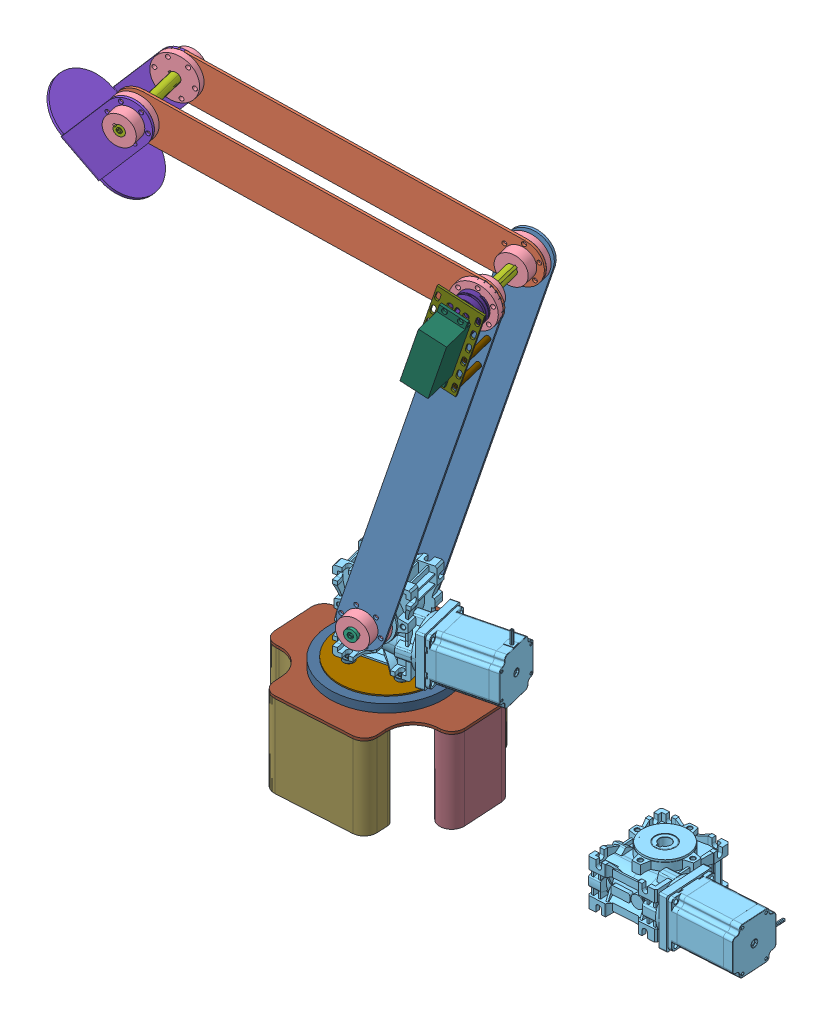
SolidWorks assembly Arm Assembly3, configuration Default. Lengths in mm.
Overall size (779.26 703.08 241.12).
36 component instances, 18 part files, 93 mates.
Components (placement in the parent):
- Link 2-1: Link 2 [Default] at (46.1352 312.2794 295.2766) x (0.282774 0.956671 -0.069421) z (0.238421 0 0.971162) size (457.2 50.8 3.17)
- Link 3-1: Link 3 [Default] at (163.2817 733.3082 355.8444) x (-0.949822 0.208481 0.233182) z (0.238421 0 0.971162) size (406.4 50.8 3.17)
- Flanged Bearing-1: Flanged Bearing [Default] at (-195.532 782.6022 375.2024) x (0.971162 0 -0.238421) z (0.238421 0 0.971162) size (38.1 38.1 12.7)
- Keyed hub-1: Keyed hub [Default] at (41.8754 319.6751 379.8434) x (0.219652 -0.974087 -0.053925) z (-0.945996 -0.226174 0.232242) size (50.8 25.4 50.8)
- Link 2-2: Link 2 [Default] at (67.3665 312.2794 381.7585) x (0.282774 0.956671 -0.069421) z (0.238421 0 0.971162) size (457.2 50.8 3.17)
- Link 3-2: Link 3 [Default] at (146.5923 733.3082 287.863) x (-0.949822 0.208481 0.233182) z (0.238421 0 0.971162) size (406.4 50.8 3.17)
- Flanged Bearing-3: Flanged Bearing [Default] at (-179.6358 782.6022 439.9523) x (-0.897412 -0.382247 0.220315) z (-0.238421 0 -0.971162) size (38.1 38.1 12.7)
- Keyed hub-2: Keyed hub [Default] at (139.5571 708.4663 281.417) x (0.721336 -0.669563 -0.177088) z (-0.650254 -0.742755 0.159638) size (50.8 25.4 50.8)
- Keyed hub-3: Keyed hub [Default] at (25.1859 319.6751 311.8621) x (-0.219652 0.974087 0.053925) z (-0.945996 -0.226174 0.232242) size (50.8 25.4 50.8)
- Keyed hub-4: Keyed hub [Default] at (160.7885 708.4663 367.8989) x (-0.721336 0.669563 0.177088) z (-0.650254 -0.742755 0.159638) size (50.8 25.4 50.8)
- Flanged Bearing-4: Flanged Bearing [Default] at (137.4376 708.4663 272.7833) x (0.894281 0.38995 -0.219546) z (-0.238421 0 -0.971162) size (38.1 38.1 12.7)
- Nema Stepper Motor-2: Nema Stepper Motor [Default] at (106.1749 300.7059 328.0186) x (0.971162 0 -0.238421) z (-0.238421 0 -0.971162) size (171.01 100.01 63.01)
- Nema Stepper Motor-3: Nema Stepper Motor [Default] at (426.1519 175.0272 335.1941) x (0.998228 0 -0.059501) z (0 -1 0) size (171.01 100.01 63.01)
- Keyed Drive Shaft-1: Keyed Drive Shaft [Default] at (6.1532 318.2181 219.9234) x (0.219652 -0.974087 -0.053925) z (0.238421 0 0.971162) size (19.9 19.9 128.01)
- Keyed Shaft-1: Keyed Shaft [Default] at (134.2192 708.4663 259.6738) x (0.721336 -0.669563 -0.177088) z (0.238421 0 0.971162) size (12.7 12.5 104.14)
- Link 4-1: Link 4 [Default] at (-253.3947 740.7663 432.1282) x (0.238421 0 0.971162) z (-0.736623 0.651677 0.180841) size (90.37 102.6 133.86)
- Keyed hub-5: Keyed hub [Default] at (-193.7642 782.6022 382.403) x (-0.632884 -0.758496 0.155373) z (0.736623 -0.651677 -0.180841) size (50.8 25.4 50.8)
- Keyed hub-6: Keyed hub [Default] at (-177.5163 782.6022 448.5859) x (0.632884 0.758496 -0.155373) z (0.736623 -0.651677 -0.180841) size (50.8 25.4 50.8)
- Keyed Shaft-2: Keyed Shaft [Default] at (-169.0381 782.6022 483.1205) x (-0.632884 -0.758496 0.155373) z (-0.238421 0 -0.971162) size (12.7 12.5 104.14)
- Bearing maybe-1: Bearing maybe [Default] at (32.1724 257.1751 346.1862) x (0.971162 0 -0.238421) z (0.238421 0 0.971162) size (117.56 1.5 117.56)
- Bearing other part-1: Bearing other part [Default] at (32.1724 247.1751 346.1862) size (140 10 140)
- Top base plate-1: Top base plate [Default] at (33.5723 244.0001 346.2554) x (0.998228 0 -0.059501) z (0.059501 0 0.998228) size (222 3.17 194.94)
- arm base spacer large part-1: arm base spacer large part [Default] at (32.1724 142.4001 346.1862) x (-0.998228 0 0.059501) z (-0.059501 0 -0.998228) size (171.5 101.6 195.24)
- arm base spacer small part-1: arm base spacer small part [Default] at (130.8381 142.4001 364.6329) x (0.998228 0 -0.059501) z (0.059501 0 0.998228) size (30 101.6 78.26)
- 4 mm M6 spacer-1: 4 mm M6 spacer [94669A162] at (64.993 260.6751 360.782) x (-1 0 0) z (0 -1 0) size (13 13 4)
- 4 mm M6 spacer-2: 4 mm M6 spacer [94669A162] at (12.5502 260.6751 373.6567) x (1 0 0) z (0 -1 0) size (13 13 4)
- 4 mm M6 spacer-3: 4 mm M6 spacer [94669A162] at (54.5025 260.6751 318.0509) x (1 0 0) z (0 -1 0) size (13 13 4)
- 4 mm M6 spacer-4: 4 mm M6 spacer [94669A162] at (2.0597 260.6751 330.9256) x (1 0 0) z (0 -1 0) size (13 13 4)
- 80 kg-1: 80 kg [Default] at (150.0764 663.0869 447.9581) x (0.282774 0.956671 -0.069421) z (-0.929083 0.291171 0.22809) size (82 48 30)
- servo plate-1: servo plate [Default] at (162.6178 689.197 403.1765) x (0.282774 0.956671 -0.069421) z (-0.929083 0.291171 0.22809) size (101.6 2.54 50.8)
- 2764K312_Servomotor Precision Flexible Shaft Coupling-1: 2764K312_Servomotor Precision Flexible Shaft Coupling [2764K312] at (163.9497 708.4663 380.7754) x (0.971162 0 -0.238421) z (0.238421 0 0.971162) size (34.04 34.04 37.8)
- Flanged Bearing-5: Flanged Bearing [Default] at (158.6689 708.4663 359.2653) x (0.813188 0.54669 -0.199638) z (-0.238421 0 -0.971162) size (38.1 38.1 12.7)
- 91125A471_Female Threaded Round Standoff-1: 91125A471_Female Threaded Round Standoff [91125A471] at (125.6348 655.4184 390.0248) x (0.971162 0 -0.238421) z (0.238421 0 0.971162) size (6.35 6.35 38.54)
- 91125A471_Female Threaded Round Standoff-2: 91125A471_Female Threaded Round Standoff [91125A471] at (174.916 674.4965 378.2401) x (-0.144728 0.988833 0.035531) z (-0.238421 0 -0.971162) size (6.35 6.35 38.54)
- 91125A471_Female Threaded Round Standoff-4: 91125A471_Female Threaded Round Standoff [91125A471] at (135.1065 687.0205 388.0133) x (-0.310292 0.947584 0.076177) z (-0.238421 0 -0.971162) size (6.35 6.35 38.54)
- 91125A471_Female Threaded Round Standoff-6: 91125A471_Female Threaded Round Standoff [91125A471] at (165.6394 642.97 380.5175) x (-0.466934 0.87683 0.114633) z (-0.238421 0 -0.971162) size (6.35 6.35 38.54)
Mates (geometry in assembly coordinates):
- Concentric3: concentric aligned: cylinder of Keyed hub-1 through (43.7678 319.6751 387.552) axis (0.238421 0 0.971162) radius 17.4625; cylinder of Link 2-2 through (43.7678 319.6751 387.552) axis (0.238421 0 0.971162) radius 17.4625
- Coincident2: coincident anti-aligned: plane of Keyed hub-1 through (43.7678 319.6751 387.552) normal (0.238421 0 0.971162); plane of Link 2-2 through (43.7678 319.6751 387.552) normal (-0.238421 0 -0.971162)
- Concentric4: concentric aligned: cylinder of Keyed hub-1 through (48.3985 299.1394 386.4152) axis (0.238421 0 0.971162) radius 2.5527; cylinder of Link 2-2 through (49.1555 299.1394 389.4986) axis (0.238421 0 0.971162) radius 2.5527
- Concentric5: concentric anti-aligned: cylinder of Link 2-1 through (22.5365 319.6751 301.0701) axis (0.238421 0 0.971162) radius 17.4625; cylinder of Keyed hub-3 through (23.2934 319.6751 304.1535) axis (-0.238421 0 -0.971162) radius 17.4625
- Coincident3: coincident anti-aligned: plane of Link 2-1 through (23.2934 319.6751 304.1535) normal (0.238421 0 0.971162); plane of Keyed hub-3 through (23.2934 319.6751 304.1535) normal (-0.238421 0 -0.971162)
- Concentric7: concentric anti-aligned: cylinder of Link 2-1 through (3.7065 325.8136 308.9621) axis (0.238421 0 0.971162) radius 2.5527; cylinder of Keyed hub-3 through (3.7065 325.8136 308.9621) axis (-0.238421 0 -0.971162) radius 2.5527
- Concentric8: concentric anti-aligned: cylinder of Keyed hub-1 through (41.8754 319.6751 379.8434) axis (0.238421 0 0.971162) radius 6.35; cylinder of Keyed hub-3 through (25.1859 319.6751 311.8621) axis (-0.238421 0 -0.971162) radius 6.35
- Coincident5: coincident aligned: plane of Keyed hub-1 through (41.5267 321.2215 379.929) normal (0.219652 -0.974087 -0.053925); plane of Keyed hub-3 through (24.8372 321.2215 311.9477) normal (0.219652 -0.974087 -0.053925)
- Concentric10: concentric anti-aligned: cylinder of Link 2-1 through (137.4557 708.4663 272.8573) axis (0.238421 0 0.971162) radius 17.4625; cylinder of Flanged Bearing-4 through (135.9236 708.4663 266.6165) axis (-0.238421 0 -0.971162) radius 17.4625
- Concentric11: concentric anti-aligned: cylinder of Link 3-1 through (158.139 708.4663 357.1069) axis (0.238421 0 0.971162) radius 17.4625; cylinder of Keyed hub-4 through (158.896 708.4663 360.1903) axis (-0.238421 0 -0.971162) radius 17.4625
- Coincident8: coincident anti-aligned: plane of Link 3-1 through (158.896 708.4663 360.1903) normal (0.238421 0 0.971162); plane of Keyed hub-4 through (158.896 708.4663 360.1903) normal (-0.238421 0 -0.971162)
- Concentric12: concentric anti-aligned: cylinder of Link 3-1 through (163.1645 729.085 359.1424) axis (0.238421 0 0.971162) radius 2.5527; cylinder of Keyed hub-4 through (163.1645 729.085 359.1424) axis (-0.238421 0 -0.971162) radius 2.5527
- Concentric13: concentric aligned: cylinder of Link 3-2 through (141.4496 708.4663 289.1256) axis (0.238421 0 0.971162) radius 17.4625; cylinder of Keyed hub-2 through (141.4496 708.4663 289.1256) axis (0.238421 0 0.971162) radius 17.4625
- Coincident9: coincident anti-aligned: plane of Link 3-2 through (141.4496 708.4663 289.1256) normal (-0.238421 0 -0.971162); plane of Keyed hub-2 through (141.4496 708.4663 289.1256) normal (0.238421 0 0.971162)
- Concentric14: concentric aligned: cylinder of Link 3-2 through (146.475 729.085 291.1611) axis (0.238421 0 0.971162) radius 2.5527; cylinder of Keyed hub-2 through (145.718 729.085 288.0777) axis (0.238421 0 0.971162) radius 2.5527
- Concentric15: concentric anti-aligned: cylinder of Keyed hub-2 through (139.5571 708.4663 281.417) axis (0.238421 0 0.971162) radius 6.35; cylinder of Keyed hub-4 through (160.7885 708.4663 367.8989) axis (-0.238421 0 -0.971162) radius 6.35
- Coincident10: coincident aligned: plane of Keyed hub-2 through (140.7022 707.4034 281.1358) normal (-0.721336 0.669563 0.177088); plane of Keyed hub-4 through (161.9336 707.4034 367.6178) normal (-0.721336 0.669563 0.177088)
- Concentric17: concentric aligned: cylinder of Flanged Bearing-1 through (-194.018 782.6022 381.3693) axis (0.238421 0 0.971162) radius 17.4625; cylinder of Link 3-2 through (-196.3071 782.6022 372.045) axis (0.238421 0 0.971162) radius 17.4625
- Coincident13: coincident anti-aligned: plane of Flanged Bearing-1 through (-196.3071 800.0647 372.045) normal (0.238421 0 0.971162); plane of Link 3-2 through (141.4496 708.4663 289.1256) normal (-0.238421 0 -0.971162)
- Concentric18: concentric anti-aligned: cylinder of Link 3-1 through (-179.6177 782.6022 440.0263) axis (0.238421 0 0.971162) radius 17.4625; cylinder of Flanged Bearing-3 through (-181.1498 782.6022 433.7854) axis (-0.238421 0 -0.971162) radius 17.4625
- Coincident14: coincident anti-aligned: plane of Link 3-1 through (158.896 708.4663 360.1903) normal (0.238421 0 0.971162); plane of Flanged Bearing-3 through (-185.3432 798.7386 444.7012) normal (-0.238421 0 -0.971162)
- Concentric21: concentric anti-aligned: cylinder of Keyed hub-1 through (41.8754 319.6751 379.8434) axis (0.238421 0 0.971162) radius 6.35; cylinder of Keyed Drive Shaft-1 through (48.7896 319.6751 408.0071) axis (-0.238421 0 -0.971162) radius 7
- Parallel1: parallel anti-aligned: plane of Keyed hub-1 through (41.5267 321.2215 379.929) normal (0.219652 -0.974087 -0.053925); plane of Keyed Drive Shaft-1 through (37.9953 323.3091 344.7567) normal (-0.219652 0.974087 0.053925)
- Coincident18: coincident anti-aligned: plane of Keyed hub-3 through (25.1859 319.6751 311.8621) normal (0.238421 0 0.971162); plane of Keyed Drive Shaft-1 through (31.2541 322.3579 310.3723) normal (-0.238421 0 -0.971162)
- Coincident19: coincident anti-aligned: plane of Keyed hub-1 through (41.8754 319.6751 379.8434) normal (-0.238421 0 -0.971162); plane of Keyed Drive Shaft-1 through (47.9436 322.3579 378.3537) normal (0.238421 0 0.971162)
- Concentric22: concentric anti-aligned: cylinder of Keyed hub-2 through (139.5571 708.4663 281.417) axis (0.238421 0 0.971162) radius 6.35; cylinder of Keyed Shaft-1 through (161.4707 708.4663 370.6776) axis (-0.238421 0 -0.971162) radius 6.35
- Coincident20: coincident aligned: plane of Keyed hub-2 through (140.7022 707.4034 281.1358) normal (-0.721336 0.669563 0.177088); plane of Keyed Shaft-1 through (165.7044 710.9313 369.6383) normal (-0.721336 0.669563 0.177088)
- Coincident22: coincident anti-aligned: plane of Link 2-1 through (23.2934 319.6751 304.1535) normal (0.238421 0 0.971162); plane of Flanged Bearing-4 through (144.8259 692.3862 274.3172) normal (-0.238421 0 -0.971162)
- Distance1: distance = 2.54 mm anti-aligned: plane of Flanged Bearing-4 through (143.309 697.871 277.8805) normal (0.238421 0 0.971162); plane of Keyed hub-2 through (139.5571 708.4663 281.417) normal (-0.238421 0 -0.971162)
- Concentric23: concentric anti-aligned: cylinder of Link 4-1 through (-174.8668 782.6022 459.378) axis (-0.238421 0 -0.971162) radius 17.4625; cylinder of Keyed hub-6 through (-175.6238 782.6022 456.2945) axis (0.238421 0 0.971162) radius 17.4625
- Concentric24: concentric anti-aligned: cylinder of Link 4-1 through (-182.4015 802.4955 457.9585) axis (-0.238421 0 -0.971162) radius 2.5527; cylinder of Keyed hub-6 through (-182.4015 802.4955 457.9585) axis (0.238421 0 0.971162) radius 2.5527
- Coincident27: coincident anti-aligned: plane of Link 4-1 through (-269.3354 709.6572 479.3008) normal (-0.238421 0 -0.971162); plane of Keyed hub-6 through (-175.6238 782.6022 456.2945) normal (0.238421 0 0.971162)
- Concentric25: concentric anti-aligned: cylinder of Link 4-1 through (-196.4137 782.6022 371.611) axis (0.238421 0 0.971162) radius 17.4625; cylinder of Keyed hub-5 through (-195.6567 782.6022 374.6944) axis (-0.238421 0 -0.971162) radius 17.4625
- Concentric26: concentric anti-aligned: cylinder of Link 4-1 through (-202.4344 802.4955 376.3583) axis (0.238421 0 0.971162) radius 2.5527; cylinder of Keyed hub-5 through (-202.4344 802.4955 376.3583) axis (-0.238421 0 -0.971162) radius 2.5527
- Concentric27: concentric anti-aligned: cylinder of Keyed hub-5 through (-193.7642 782.6022 382.403) axis (-0.238421 0 -0.971162) radius 6.35; cylinder of Keyed Shaft-2 through (-196.2895 782.6022 372.1167) axis (0.238421 0 0.971162) radius 6.35
- Coincident31: coincident aligned: plane of Keyed hub-5 through (-192.7595 783.8063 382.1563) normal (-0.632884 -0.758496 0.155373); plane of Keyed Shaft-2 through (-198.7836 786.9016 372.729) normal (-0.632884 -0.758496 0.155373)
- Coincident32: coincident aligned: plane of Keyed hub-6 through (-171.4604 782.6022 473.2535) normal (0.238421 0 0.971162); plane of Keyed Shaft-2 through (-171.4604 782.6022 473.2535) normal (0.238421 0 0.971162)
- Coincident34: coincident anti-aligned: plane of Link 4-1 through (-289.3683 709.6572 397.7006) normal (0.238421 0 0.971162); plane of Keyed hub-5 through (-195.6567 782.6022 374.6944) normal (-0.238421 0 -0.971162)
- Coincident36: coincident aligned: plane of Keyed hub-6 through (-178.521 781.3981 448.8326) normal (0.632884 0.758496 -0.155373); plane of Keyed Shaft-2 through (-200.793 784.4934 373.2223) normal (0.632884 0.758496 -0.155373)
- Concentric28: concentric anti-aligned: cone of Flanged Bearing-3 through (-178.2815 782.6022 445.4689) axis (-0.238421 0 -0.971162); cylinder of Keyed Shaft-2 through (-196.2895 782.6022 372.1167) axis (0.238421 0 0.971162) radius 6.35
- Distance3: distance = 2.54 mm anti-aligned: plane of Flanged Bearing-3 through (-182.3933 793.2346 447.1678) normal (0.238421 0 0.971162); plane of Keyed hub-6 through (-177.5163 782.6022 448.5859) normal (-0.238421 0 -0.971162)
- Coincident37: coincident anti-aligned: plane of Bearing maybe-1 through (32.1724 257.1751 346.1862) normal (0 -1 0); plane of Bearing other part-1 through (32.1724 257.1751 346.1862) normal (0 1 0)
- Concentric29: concentric aligned: cylinder of Bearing maybe-1 through (32.1724 258.6751 346.1862) axis (0 -1 0) radius 58.7822; cylinder of Bearing other part-1 through (32.1724 257.1751 346.1862) axis (0 -1 0) radius 70
- Coincident38: coincident anti-aligned: plane of Top base plate-1 through (74.0847 244.0001 261.2257) normal (0 -1 0); plane of arm base spacer small part-1 through (130.8381 244.0001 364.6329) normal (0 1 0)
- Coincident40: coincident anti-aligned: plane of Top base plate-1 through (74.0847 244.0001 261.2257) normal (0 -1 0); plane of arm base spacer large part-1 through (32.1724 244.0001 346.1862) normal (0 1 0)
- Coincident45: coincident anti-aligned: plane of Bearing other part-1 through (32.1724 247.1751 346.1862) normal (0 -1 0); plane of Top base plate-1 through (74.0847 247.1751 261.2257) normal (0 1 0)
- Concentric32: concentric aligned: cylinder of Bearing other part-1 through (32.1724 257.1751 346.1862) axis (0 -1 0) radius 70; circle of arm base spacer large part-1
- Coincident50: coincident anti-aligned: plane of Bearing maybe-1 through (32.1724 258.6751 346.1862) normal (0 1 0); plane of 4 mm M6 spacer-3 through (54.5025 258.6751 318.0509) normal (0 -1 0)
- Coincident55: coincident anti-aligned: plane of Nema Stepper Motor-2 through (106.1749 300.7059 328.0186) normal (-0.238421 0 -0.971162); plane of Bearing maybe-1 through (32.1724 257.1751 346.1862) normal (0.238421 0 0.971162)
- Distance5: distance = 76.2 mm aligned: plane of Nema Stepper Motor-2 through (106.1749 300.7059 328.0186) normal (0.971162 0 -0.238421); plane of Bearing maybe-1 through (32.1724 257.1751 346.1862) normal (0.971162 0 -0.238421)
- Coincident57: coincident aligned: plane of Top base plate-1 through (-6.0476 247.1751 446.2586) normal (0.059501 0 0.998228); plane of arm base spacer large part-1 through (84.7912 244.0001 440.844) normal (0.059501 0 0.998228)
- Coincident58: coincident aligned: plane of Top base plate-1 through (-75.7951 247.1751 376.9496) normal (-0.998228 0 0.059501); plane of arm base spacer large part-1 through (-75.8042 244.0001 376.7975) normal (-0.998228 0 0.059501)
- Concentric37: concentric aligned: cylinder of Top base plate-1 through (130.8381 247.1751 364.6329) axis (0 -1 0) radius 15; cylinder of arm base spacer small part-1 through (130.8381 244.0001 364.6329) axis (0 -1 0) radius 15
- Coincident59: coincident aligned: plane of Top base plate-1 through (145.8116 247.1751 363.7404) normal (0.998228 0 -0.059501); plane of arm base spacer small part-1 through (145.8116 244.0001 363.7404) normal (0.998228 0 -0.059501)
- Parallel2: parallel aligned: plane of Nema Stepper Motor-3 through (350.3499 203.0272 320.7095) normal (0 1 0); plane of Top base plate-1 through (74.0847 247.1751 261.2257) normal (0 1 0)
- Parallel3: parallel anti-aligned: plane of Nema Stepper Motor-3 through (312.2058 175.0272 353.0364) normal (-0.998228 0 0.059501); plane of arm base spacer small part-1 through (145.8116 244.0001 363.7404) normal (0.998228 0 -0.059501)
- Coincident61: coincident anti-aligned: plane of Nema Stepper Motor-2 through (79.0486 262.6751 363.5095) normal (0 -1 0); plane of 4 mm M6 spacer-1 through (64.993 262.6751 360.782) normal (0 1 0)
- Concentric39: concentric aligned: cylinder of Nema Stepper Motor-2 through (64.993 359.6751 360.782) axis (0 -1 0) radius 3.25; cylinder of 4 mm M6 spacer-1 through (64.993 262.6751 360.782) axis (0 -1 0) radius 3.15
- Coincident62: coincident anti-aligned: plane of Bearing maybe-1 through (32.1724 258.6751 346.1862) normal (0 1 0); plane of 4 mm M6 spacer-1 through (64.993 258.6751 360.782) normal (0 -1 0)
- Concentric40: concentric aligned: cylinder of Nema Stepper Motor-2 through (54.5025 359.6751 318.0509) axis (0 -1 0) radius 3.25; cylinder of 4 mm M6 spacer-3 through (54.5025 262.6751 318.0509) axis (0 -1 0) radius 3.15
- Concentric41: concentric aligned: cylinder of Nema Stepper Motor-2 through (2.0597 359.6751 330.9256) axis (0 -1 0) radius 3.25; cylinder of 4 mm M6 spacer-4 through (2.0597 262.6751 330.9256) axis (0 -1 0) radius 3.15
- Concentric42: concentric aligned: cylinder of Nema Stepper Motor-2 through (12.5502 359.6751 373.6567) axis (0 -1 0) radius 3.25; cylinder of 4 mm M6 spacer-2 through (12.5502 262.6751 373.6567) axis (0 -1 0) radius 3.15
- Concentric43: concentric aligned: cylinder of Keyed hub-1 through (43.7678 319.6751 387.552) axis (0.238421 0 0.971162) radius 17.4625; cylinder of Nema Stepper Motor-2 through (11.423 319.6751 255.8014) axis (0.238421 0 0.971162) radius 7
- Coincident65: coincident anti-aligned: plane of Nema Stepper Motor-2 through (41.0366 319.6751 376.4454) normal (0.238421 0 0.971162); plane of Keyed Drive Shaft-1 through (41.0409 319.6751 376.4444) normal (-0.238421 0 -0.971162)
- Coincident69: coincident anti-aligned: plane of 80 kg-1 through (140.4203 663.0869 408.626) normal (-0.238421 0 -0.971162); plane of servo plate-1 through (162.6178 689.197 403.1765) normal (0.238421 0 0.971162)
- Concentric48: concentric aligned: cylinder of 80 kg-1 through (175.9096 728.1613 441.616) axis (-0.238421 0 -0.971162) radius 3; cylinder of servo plate-1 through (166.2535 728.1613 402.2839) axis (-0.238421 0 -0.971162) radius 3.302
- Concentric49: concentric aligned: cylinder of 80 kg-1 through (191.704 723.2114 437.7385) axis (-0.238421 0 -0.971162) radius 3; cylinder of servo plate-1 through (182.048 723.2114 398.4064) axis (-0.238421 0 -0.971162) radius 3.302
- Concentric50: concentric aligned: cylinder of 80 kg-1 through (154.7016 656.411 446.8226) axis (-0.238421 0 -0.971162) radius 3; cylinder of servo plate-1 through (145.0455 656.411 407.4905) axis (-0.238421 0 -0.971162) radius 3.302
- Concentric51: concentric aligned: cylinder of 80 kg-1 through (170.496 651.4611 442.9451) axis (-0.238421 0 -0.971162) radius 3; cylinder of servo plate-1 through (160.8399 651.4611 403.613) axis (-0.238421 0 -0.971162) radius 3.302
- Coincident71: coincident anti-aligned: plane of Link 2-2 through (44.5248 319.6751 390.6355) normal (0.238421 0 0.971162); plane of 2764K312_Servomotor Precision Flexible Shaft Coupling-1 through (159.4441 708.4663 362.4227) normal (-0.238421 0 -0.971162)
- Concentric53: concentric anti-aligned: cylinder of Keyed Shaft-1 through (161.4707 708.4663 370.6776) axis (-0.238421 0 -0.971162) radius 6.35; cylinder of 2764K312_Servomotor Precision Flexible Shaft Coupling-1 through (159.4441 708.4663 362.4227) axis (0.238421 0 0.971162) radius 6.35
- Concentric54: concentric anti-aligned: cylinder of 80 kg-1 through (167.2727 708.4663 394.311) axis (0.238421 0 0.971162) radius 2; cylinder of 2764K312_Servomotor Precision Flexible Shaft Coupling-1 through (168.4552 708.4663 399.128) axis (-0.238421 0 -0.971162) radius 3.175
- Concentric55: concentric aligned: cone of Flanged Bearing-4 through (138.7919 708.4663 278.2999) axis (-0.238421 0 -0.971162); cylinder of Keyed Shaft-1 through (161.4707 708.4663 370.6776) axis (-0.238421 0 -0.971162) radius 6.35
- Concentric57: concentric anti-aligned: cylinder of Keyed Shaft-1 through (161.4707 708.4663 370.6776) axis (-0.238421 0 -0.971162) radius 6.35; cylinder of 2764K312_Servomotor Precision Flexible Shaft Coupling-1 through (159.4441 708.4663 362.4227) axis (0.238421 0 0.971162) radius 6.35
- Coincident73: coincident anti-aligned: plane of Keyed Shaft-1 through (161.4707 708.4663 370.6776) normal (0.238421 0 0.971162); plane of 2764K312_Servomotor Precision Flexible Shaft Coupling-1 through (164.1127 680.0523 370.029) normal (-0.238421 0 -0.971162)
- Concentric58: concentric anti-aligned: cylinder of Link 2-2 through (158.6871 708.4663 359.3393) axis (0.238421 0 0.971162) radius 17.4625; cylinder of Flanged Bearing-5 through (157.155 708.4663 353.0984) axis (-0.238421 0 -0.971162) radius 17.4625
- Coincident74: coincident anti-aligned: plane of Link 2-2 through (44.5248 319.6751 390.6355) normal (0.238421 0 0.971162); plane of Flanged Bearing-5 through (168.7154 693.8443 360.1466) normal (-0.238421 0 -0.971162)
- Distance6: distance = 2.54 mm aligned: plane of Flanged Bearing-5 through (166.2918 698.8317 363.9324) normal (0.238421 0 0.971162); plane of Keyed hub-4 through (160.7885 708.4663 367.8989) normal (0.238421 0 0.971162)
- Concentric59: concentric aligned: cylinder of Keyed Shaft-1 through (161.4707 708.4663 370.6776) axis (-0.238421 0 -0.971162) radius 6.35; cone of Flanged Bearing-5 through (160.0232 708.4663 364.7819) axis (-0.238421 0 -0.971162)
- Coincident75: coincident anti-aligned: plane of servo plate-1 through (162.0122 689.197 400.7098) normal (-0.238421 0 -0.971162); plane of 2764K312_Servomotor Precision Flexible Shaft Coupling-1 through (168.4552 708.4663 399.128) normal (0.238421 0 0.971162)
- Parallel7: parallel anti-aligned: line of Link 2-2 through (68.1235 312.2794 384.842) axis (0.282774 0.956671 -0.069421); line of servo plate-1 through (199.9758 730.4002 391.3897) axis (-0.282774 -0.956671 0.069421)
- Coincident76: coincident anti-aligned: plane of servo plate-1 through (162.0122 689.197 400.7098) normal (-0.238421 0 -0.971162); plane of 91125A471_Female Threaded Round Standoff-1 through (130.1767 655.4184 408.5254) normal (0.238421 0 0.971162)
- Coincident77: coincident anti-aligned: plane of Link 2-2 through (44.5248 319.6751 390.6355) normal (0.238421 0 0.971162); plane of 91125A471_Female Threaded Round Standoff-2 through (170.3741 674.4965 359.7394) normal (-0.238421 0 -0.971162)
- Coincident78: coincident anti-aligned: plane of Link 2-2 through (44.5248 319.6751 390.6355) normal (0.238421 0 0.971162); plane of 91125A471_Female Threaded Round Standoff-4 through (130.5646 687.0205 369.5127) normal (-0.238421 0 -0.971162)
- Coincident79: coincident anti-aligned: plane of Link 2-2 through (44.5248 319.6751 390.6355) normal (0.238421 0 0.971162); plane of 91125A471_Female Threaded Round Standoff-6 through (161.0975 642.97 362.0168) normal (-0.238421 0 -0.971162)
- Parallel8: parallel anti-aligned: cylinder of 91125A471_Female Threaded Round Standoff-1 through (130.1767 655.4184 408.5254) axis (-0.238421 0 -0.971162) radius 3.175; cylinder of 91125A471_Female Threaded Round Standoff-6 through (161.0975 642.97 362.0168) axis (0.238421 0 0.971162) radius 3.175
- Parallel9: parallel aligned: cylinder of 91125A471_Female Threaded Round Standoff-2 through (170.3741 674.4965 359.7394) axis (0.238421 0 0.971162) radius 3.175; cylinder of 91125A471_Female Threaded Round Standoff-4 through (130.5646 687.0205 369.5127) axis (0.238421 0 0.971162) radius 3.175
- Parallel10: parallel anti-aligned: cylinder of 91125A471_Female Threaded Round Standoff-1 through (130.1767 655.4184 408.5254) axis (-0.238421 0 -0.971162) radius 3.175; cylinder of 91125A471_Female Threaded Round Standoff-4 through (130.5646 687.0205 369.5127) axis (0.238421 0 0.971162) radius 3.175
- Parallel11: parallel aligned: cylinder of 91125A471_Female Threaded Round Standoff-2 through (170.3741 674.4965 359.7394) axis (0.238421 0 0.971162) radius 3.175; cylinder of 91125A471_Female Threaded Round Standoff-6 through (161.0975 642.97 362.0168) axis (0.238421 0 0.971162) radius 3.175
- Concentric61: concentric anti-aligned: cylinder of Link 2-2 through (161.1277 642.97 362.1402) axis (-0.238421 0 -0.971162) radius 1.972; cylinder of 91125A471_Female Threaded Round Standoff-6 through (161.0975 642.97 362.0168) axis (0.238421 0 0.971162) radius 3.175
- Concentric62: concentric anti-aligned: cylinder of Link 2-2 through (170.4044 674.4965 359.8628) axis (-0.238421 0 -0.971162) radius 1.972; cylinder of 91125A471_Female Threaded Round Standoff-2 through (170.3741 674.4965 359.7394) axis (0.238421 0 0.971162) radius 3.175
- Concentric63: concentric anti-aligned: cylinder of Link 2-2 through (130.5949 687.0205 369.636) axis (-0.238421 0 -0.971162) radius 1.972; cylinder of 91125A471_Female Threaded Round Standoff-4 through (130.5646 687.0205 369.5127) axis (0.238421 0 0.971162) radius 3.175
- Concentric64: concentric aligned: cylinder of Link 2-2 through (121.1958 655.4184 371.9435) axis (-0.238421 0 -0.971162) radius 1.972; cylinder of 91125A471_Female Threaded Round Standoff-1 through (130.1767 655.4184 408.5254) axis (-0.238421 0 -0.971162) radius 3.175
